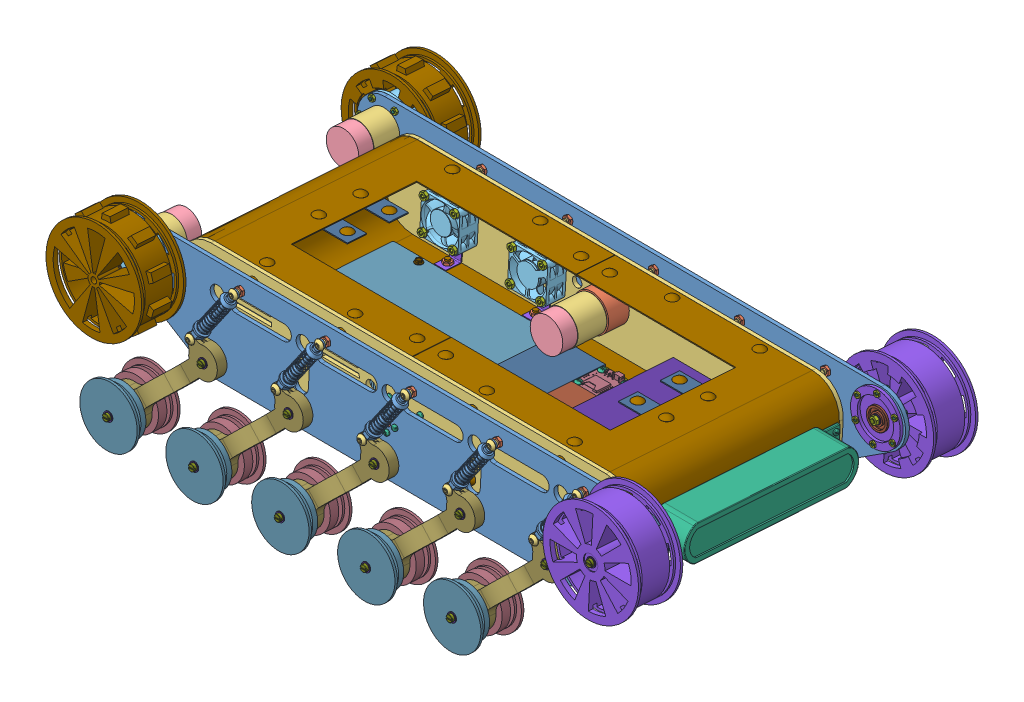
SolidWorks assembly Ensamble_Detallado_2, configuration Predeterminado. Lengths in mm. (continued)
Mates (geometry in assembly coordinates): (continued)
- Coincidente9464: coincident anti-aligned: plane of Perfil_IzquierdoV2.2-1 through (258.4555 -33.6114 -539.3761) normal (0.005872 -0.060029 -0.998179); plane of Acople-1 through (68.465 -3.1497 -542.3256) normal (-0.005872 0.060029 0.998179)
- Concéntrica118160: concentric aligned: cylinder of Perfil_IzquierdoV2.2-1 through (76.4414 -2.9112 -538.2857) axis (0.005872 -0.060029 -0.998179) radius 1.5; cylinder of Acople-1 through (76.4179 -2.6711 -534.293) axis (0.005872 -0.060029 -0.998179) radius 1.5
- Distancia1: distance = 0.55 mm anti-aligned: plane of Motor_4-2/Motor_1-1 through (68.5387 -3.9031 -554.8528) normal (-0.005872 0.060029 0.998179); plane of Acople-1 through (68.5355 -3.8701 -554.3038) normal (0.005872 -0.060029 -0.998179)
- Concéntrica118161: concentric aligned: cylinder of Motor_4-2/Motor_1-1 through (68.5387 -3.9031 -554.8528) axis (0.005872 -0.060029 -0.998179) radius 6; cylinder of Pared_chasis-2 through (68.5504 -4.0231 -556.8491) axis (0.005872 -0.060029 -0.998179) radius 6
- Coincidente9466: coincident anti-aligned: plane of Motor_4-2/Motor_1-1 through (67.8758 2.689 -561.264) normal (-0.005872 0.060029 0.998179); plane of Pared_chasis-2 through (275.5675 -9.2966 -559.3215) normal (0.005872 -0.060029 -0.998179)
- Concéntrica118165: concentric aligned: cylinder of Perfil_IzquierdoV2.2-1 through (60.4417 -2.908 -538.38) axis (0.005872 -0.060029 -0.998179) radius 1.5; cylinder of Acople-1 through (60.4182 -2.6679 -534.3873) axis (0.005872 -0.060029 -0.998179) radius 1.5
- Concéntrica118166: concentric anti-aligned: cylinder of Pared_chasis-2 through (76.058 16.8009 -558.0573) axis (0.005872 -0.060029 -0.998179) radius 1.5; cylinder of pan head tapping screw_am-43 through (76.0451 16.9329 -555.8613) axis (-0.005872 0.060029 0.998179) radius 1.5
- Coincidente9468: coincident anti-aligned: plane of Pared_chasis-2 through (275.544 -9.0565 -555.3288) normal (-0.005872 0.060029 0.998179); plane of pan head tapping screw_am-43 through (77.4539 14.3785 -557.9034) normal (0.005872 -0.060029 -0.998179)
- Concéntrica118167: concentric anti-aligned: cylinder of Perfil_IzquierdoV2.2-1 through (76.4414 -2.9112 -538.2857) axis (0.005872 -0.060029 -0.998179) radius 1.5; cylinder of pan head tapping screw_am-44 through (76.4285 -2.7792 -536.0897) axis (-0.005872 0.060029 0.998179) radius 1.5
- Coincidente9469: coincident anti-aligned: plane of Perfil_IzquierdoV2.2-1 through (258.432 -33.3713 -535.3834) normal (-0.005872 0.060029 0.998179); plane of pan head tapping screw_am-44 through (77.8372 -5.3336 -538.1318) normal (0.005872 -0.060029 -0.998179)
- Concéntrica118168: concentric aligned: cylinder of pan head tapping screw_am-44 through (76.4285 -2.7792 -536.0897) axis (-0.005872 0.060029 0.998179) radius 1.5; cylinder of hex nut style 1_am-64 through (76.4907 -3.4155 -546.6704) axis (-0.005872 0.060029 0.998179) radius 1.25
- Coincidente9470: coincident anti-aligned: plane of Acople-1 through (68.4767 -3.2698 -544.322) normal (0.005872 -0.060029 -0.998179); plane of hex nut style 1_am-64 through (80.2996 0.6768 -544.4898) normal (-0.005872 0.060029 0.998179)
- Paralelo35: parallel aligned: plane of Perfil_IzquierdoV2.2-1 through (-191.5245 49.7885 -543.0313) normal (0.000558 0.998197 -0.060026); plane of Pared_chasis-2 through (275.5742 44.8461 -558.5702) normal (0.000558 0.998197 -0.060026)
- Concéntrica118175: concentric anti-aligned: cylinder of Acople-1 through (68.5089 1.4211 -549.613) axis (-0.000558 -0.998197 0.060026) radius 1.5; cylinder of socket set screw cup point_ai-2 through (68.516 14.0982 -550.3753) axis (0.000558 0.998197 -0.060026) radius 1.5875
- Coincidente9473: coincident anti-aligned: plane of Ensamble_internoV1.1-1/ChasisV1.7-1 through (275.5809 14.6601 -560.7622) normal (-0.005872 0.060029 0.998179); plane of Pared_chasis-2 through (275.5675 -9.2966 -559.3215) normal (0.005872 -0.060029 -0.998179)
- Coincidente9474: coincident aligned: circle of Ensamble_internoV1.1-1/ChasisV1.7-1; circle of Pared_chasis-2
- Coincidente9477: coincident anti-aligned: plane of Pieza_union_chasis-3 through (-0.4051 43.6643 -564.1299) normal (-0.005872 0.060029 0.998179); plane of Pared_chasis-2 through (275.5675 -9.2966 -559.3215) normal (0.005872 -0.060029 -0.998179)
- Concéntrica118176: concentric aligned: circle of Pieza_union_chasis-3; cylinder of Pared_chasis-2 through (-0.4635 32.2862 -553.4277) axis (0.005872 -0.060029 -0.998179) radius 2.5
- Concéntrica118177: concentric anti-aligned: cylinder of round head bolt_ai-12 through (-0.4438 32.0846 -556.78) axis (-0.005872 0.060029 0.998179) radius 2.413; cylinder of Pared_chasis-2 through (-0.4635 32.2862 -553.4277) axis (0.005872 -0.060029 -0.998179) radius 2.5
- Coincidente9479: coincident anti-aligned: plane of round head bolt_ai-12 through (5.3374 31.9281 -559.383) normal (0.005872 -0.060029 -0.998179); plane of Pared_chasis-2 through (275.544 -9.0565 -555.3288) normal (-0.005872 0.060029 0.998179)
- Concéntrica118179: concentric anti-aligned: cylinder of hex nut jam_am-22 through (161.6055 -26.9975 -661.0978) axis (-0.000136 -0.06003 -0.998197) radius 2.1; cylinder of Pieza_union_chasis-9 through (-0.3972 -26.5933 -560.9065) axis (-0.005872 0.060029 0.998179) radius 2.5
- Coincidente9484: coincident anti-aligned: plane of Pared_chasis-2 through (275.5675 -9.2966 -559.3215) normal (0.005872 -0.060029 -0.998179); plane of Pieza_union_chasis-7 through (229.5909 43.6172 -562.7741) normal (-0.005872 0.060029 0.998179)
- Concéntrica118183: concentric anti-aligned: cylinder of Pared_chasis-2 through (229.5325 32.2391 -552.072) axis (0.005872 -0.060029 -0.998179) radius 2.5; cylinder of Pieza_union_chasis-7 through (229.5971 31.5788 -563.0519) axis (-0.005872 0.060029 0.998179) radius 2.5
- Concéntrica118184: concentric anti-aligned: cylinder of Ensamble_internoV1.1-1/ChasisV1.7-1 through (229.6462 -39.8004 -566.7736) axis (-0.000029 0.998197 -0.06003) radius 2.5; cylinder of Pieza_union_chasis-7 through (229.6435 50.0643 -572.1779) axis (0.000029 -0.998197 0.06003) radius 2.5
- Coincidente9485: coincident anti-aligned: plane of hex nut jam_am-33 through (229.9097 26.979 -562.7735) normal (-0.005872 0.060029 0.998179); plane of Pieza_union_chasis-7 through (229.5967 43.5572 -563.7723) normal (0.005872 -0.060029 -0.998179)
- Concéntrica118185: concentric aligned: cylinder of Pared_chasis-2 through (229.5325 32.2391 -552.072) axis (0.005872 -0.060029 -0.998179) radius 2.5; cylinder of hex nut jam_am-33 through (229.5971 31.5788 -563.0519) axis (0.005872 -0.060029 -0.998179) radius 2.1
- Coincidente9486: coincident anti-aligned: plane of Pared_chasis-2 through (275.544 -9.0565 -555.3288) normal (-0.005872 0.060029 0.998179); plane of round head bolt_ai-33 through (235.3334 31.881 -558.0272) normal (0.005872 -0.060029 -0.998179)
- Concéntrica118186: concentric anti-aligned: cylinder of Pared_chasis-2 through (229.5325 32.2391 -552.072) axis (0.005872 -0.060029 -0.998179) radius 2.5; cylinder of round head bolt_ai-33 through (229.5522 32.0375 -555.4242) axis (-0.005872 0.060029 0.998179) radius 2.413
- Coincidente9487: coincident anti-aligned: plane of Ensamble_internoV1.1-1/ChasisV1.7-1 through (-137.1798 31.8418 -774.6065) normal (-0.000029 0.998197 -0.06003); plane of round head bolt_ai-32 through (235.4095 44.0483 -571.8161) normal (0.000029 -0.998197 0.06003)
- Concéntrica118187: concentric aligned: cylinder of Ensamble_internoV1.1-1/ChasisV1.7-1 through (229.6462 -39.8004 -566.7736) axis (-0.000029 0.998197 -0.06003) radius 2.5; cylinder of round head bolt_ai-32 through (229.6436 46.685 -571.9747) axis (-0.000029 0.998197 -0.06003) radius 2.413
- Coincidente9488: coincident anti-aligned: plane of hex nut jam_am-32 through (229.9564 41.8021 -576.2976) normal (-0.000029 0.998197 -0.06003); plane of Pieza_union_chasis-7 through (235.6906 41.6008 -579.648) normal (0.000029 -0.998197 0.06003)
- Concéntrica118188: concentric aligned: cylinder of round head bolt_ai-32 through (229.6436 46.685 -571.9747) axis (-0.000029 0.998197 -0.06003) radius 2.413; cylinder of hex nut jam_am-32 through (229.6438 39.3836 -571.5356) axis (-0.000029 0.998197 -0.06003) radius 2.1
- Tangente1: tangent aligned: cylinder of Acople-1 through (68.5355 -3.8701 -554.3038) axis (-0.005872 0.060029 0.998179) radius 5; plane of socket set screw cup point_ai-2 through (68.5089 1.4211 -549.613) normal (0.000558 0.998197 -0.060026)
- Coincidente9489: coincident anti-aligned: plane of Ensamble_internoV1.1-1/ChasisV1.7-1 through (306.8142 -21.8912 -768.7633) normal (0.999983 0.000382 0.005859); plane of Soporte_zed-1 through (305.7303 18.7868 -586.4375) normal (-0.999983 -0.000382 -0.005859)
- Concéntrica118193: concentric anti-aligned: cylinder of Soporte_zed-1 through (308.6187 9.2915 -566.7568) axis (-0.999983 -0.000382 -0.005859) radius 1.5; cylinder of pan head tapping screw_am-57 through (310.8186 9.2924 -566.7439) axis (0.999983 0.000382 0.005859) radius 1.5
- Coincidente9492: coincident anti-aligned: plane of Soporte_zed-1 through (308.7833 0.6233 -594.2856) normal (0.999983 0.000382 0.005859); plane of pan head tapping screw_am-57 through (308.6257 11.7436 -568.1086) normal (-0.999983 -0.000382 -0.005859)
- Concéntrica118194: concentric anti-aligned: cylinder of Soporte_zed-1 through (308.6191 -4.6832 -565.9164) axis (-0.999983 -0.000382 -0.005859) radius 1.5; cylinder of pan head tapping screw_am-56 through (310.819 -4.6824 -565.9035) axis (0.999983 0.000382 0.005859) radius 1.5
- Coincidente9493: coincident anti-aligned: plane of Soporte_zed-1 through (308.7833 0.6233 -594.2856) normal (0.999983 0.000382 0.005859); plane of pan head tapping screw_am-56 through (308.6261 -2.2312 -567.2682) normal (-0.999983 -0.000382 -0.005859)
- Concéntrica118195: concentric anti-aligned: cylinder of Soporte_zed-1 through (309.7754 -2.5341 -763.3981) axis (-0.999983 -0.000382 -0.005859) radius 1.5; cylinder of pan head tapping screw_am-55 through (311.9754 -2.5333 -763.3853) axis (0.999983 0.000382 0.005859) radius 1.5
- Coincidente9494: coincident anti-aligned: plane of Soporte_zed-1 through (309.6112 -7.8407 -735.0289) normal (0.999983 0.000382 0.005859); plane of pan head tapping screw_am-55 through (309.7824 -0.0821 -764.7499) normal (-0.999983 -0.000382 -0.005859)
- Concéntrica118196: concentric anti-aligned: cylinder of Soporte_zed-1 through (309.7758 -16.5089 -762.5577) axis (-0.999983 -0.000382 -0.005859) radius 1.5; cylinder of pan head tapping screw_am-54 through (311.9758 -16.5081 -762.5448) axis (0.999983 0.000382 0.005859) radius 1.5
- Coincidente9495: coincident aligned: plane of Soporte_zed-1 through (309.6112 -7.8407 -735.0289) normal (0.999983 0.000382 0.005859); circle of pan head tapping screw_am-54
- Concéntrica118197: concentric anti-aligned: cylinder of pan head tapping screw_am-57 through (310.8186 9.2924 -566.7439) axis (0.999983 0.000382 0.005859) radius 1.5; cylinder of hex nut style 1_am-70 through (304.6187 9.29 -566.7802) axis (-0.999983 -0.000382 -0.005859) radius 1.25
- Coincidente9496: coincident anti-aligned: plane of Ensamble_internoV1.1-1/ChasisV1.7-1 through (305.8142 -21.8916 -768.7692) normal (-0.999983 -0.000382 -0.005859); plane of hex nut style 1_am-70 through (304.6117 4.0092 -565.243) normal (0.999983 0.000382 0.005859)
- Concéntrica118198: concentric anti-aligned: cylinder of pan head tapping screw_am-56 through (310.819 -4.6824 -565.9035) axis (0.999983 0.000382 0.005859) radius 1.5; cylinder of hex nut style 1_am-71 through (304.6192 -4.6848 -565.9398) axis (-0.999983 -0.000382 -0.005859) radius 1.25
- Coincidente9497: coincident anti-aligned: plane of Ensamble_internoV1.1-1/ChasisV1.7-1 through (305.8142 -21.8916 -768.7692) normal (-0.999983 -0.000382 -0.005859); plane of hex nut style 1_am-71 through (304.6122 -9.9656 -564.4025) normal (0.999983 0.000382 0.005859)
- Concéntrica118199: concentric anti-aligned: cylinder of pan head tapping screw_am-55 through (311.9754 -2.5333 -763.3853) axis (0.999983 0.000382 0.005859) radius 1.5; cylinder of hex nut style 1_am-68 through (305.7755 -2.5357 -763.4216) axis (-0.999983 -0.000382 -0.005859) radius 1.25
- Coincidente9498: coincident anti-aligned: plane of Ensamble_internoV1.1-1/ChasisV1.7-1 through (305.8142 -21.8916 -768.7692) normal (-0.999983 -0.000382 -0.005859); plane of hex nut style 1_am-68 through (305.7685 -7.8165 -761.8843) normal (0.999983 0.000382 0.005859)
- Concéntrica118200: concentric anti-aligned: cylinder of pan head tapping screw_am-54 through (311.9758 -16.5081 -762.5448) axis (0.999983 0.000382 0.005859) radius 1.5; cylinder of hex nut style 1_am-69 through (305.7759 -16.5104 -762.5812) axis (-0.999983 -0.000382 -0.005859) radius 1.25
- Coincidente9499: coincident anti-aligned: plane of Ensamble_internoV1.1-1/ChasisV1.7-1 through (305.8142 -21.8916 -768.7692) normal (-0.999983 -0.000382 -0.005859); plane of hex nut style 1_am-69 through (305.7689 -21.7912 -761.0439) normal (0.999983 0.000382 0.005859)
- Coincidente9501: coincident anti-aligned: plane of Ensamble_internoV1.1-1/ChasisV1.7-1 through (306.8142 -21.8912 -768.7633) normal (0.999983 0.000382 0.005859); plane of ZED.step-3 through (305.7833 0.6222 -594.3032) normal (-0.999983 -0.000382 -0.005859)
- Concéntrica118201: concentric aligned: cylinder of Soporte_zed-1 through (306.6112 -7.8419 -735.0465) axis (0.999983 0.000382 0.005859) radius 17; cone of ZED.step-3 through (306.5112 -7.8419 -735.0471) axis (0.999983 0.000382 0.005859)
- Concéntrica118202: concentric aligned: cylinder of Soporte_zed-1 through (305.7833 0.6222 -594.3032) axis (0.999983 0.000382 0.005859) radius 17; cone of ZED.step-3 through (305.6833 0.6221 -594.3038) axis (0.999983 0.000382 0.005859)
- Concéntrica118203: concentric aligned: cylinder of Soporte_zed-1 through (306.6112 -7.8419 -735.0465) axis (0.999983 0.000382 0.005859) radius 17; cylinder of Tapazed-1 through (338.0107 -7.8299 -734.8625) axis (0.999983 0.000382 0.005859) radius 17
- Concéntrica118204: concentric aligned: cylinder of Soporte_zed-1 through (305.7833 0.6222 -594.3032) axis (0.999983 0.000382 0.005859) radius 17; cylinder of Tapazed-1 through (337.1828 0.6342 -594.1192) axis (0.999983 0.000382 0.005859) radius 17
- Coincidente9503: coincident anti-aligned: plane of ZED.step-3 through (338.0107 -7.8299 -734.8625) normal (0.999983 0.000382 0.005859); plane of Tapazed-1 through (337.1349 15.8796 -586.9451) normal (-0.999983 -0.000382 -0.005859)
- Concéntrica1182071: concentric aligned: cylinder of fan-1 through (16.1953 17.9752 -582.5238) axis (-0.005872 0.060029 0.998179) radius 2; cylinder of fillister head tapping screw_ai-1 through (16.0403 19.5593 -556.1843) axis (-0.005872 0.060029 0.998179) radius 1.9177
- Concéntrica118208: concentric aligned: cylinder of fan-1 through (-15.8042 17.9696 -582.7117) axis (-0.005872 0.060029 0.998179) radius 2; cylinder of fillister head tapping screw_ai-2 through (-15.9591 19.5536 -556.3721) axis (-0.005872 0.060029 0.998179) radius 1.9177
- Concéntrica118209: concentric aligned: cylinder of fan-1 through (-15.8098 -13.9727 -580.7908) axis (-0.005872 0.060029 0.998179) radius 2; cylinder of fillister head tapping screw_ai-6 through (-15.9647 -12.3887 -554.4512) axis (-0.005872 0.060029 0.998179) radius 1.9177
- Concéntrica118210: concentric aligned: cylinder of fan-1 through (16.1896 -13.967 -580.6029) axis (-0.005872 0.060029 0.998179) radius 2; cylinder of fillister head tapping screw_ai-7 through (16.0347 -12.383 -554.2633) axis (-0.005872 0.060029 0.998179) radius 1.9177
- Coincidente9506: coincident anti-aligned: plane of fan-1 through (16.1896 -13.967 -580.6029) normal (0.005872 -0.060029 -0.998179); plane of hex nut style 1 gradeab_bsi-7 through (16.9128 21.9456 -582.7584) normal (-0.005872 0.060029 0.998179)
- Concéntrica118211: concentric anti-aligned: cylinder of hex nut style 1 gradeab_bsi-7 through (16.1953 17.9752 -582.5238) axis (0.005872 -0.060029 -0.998179) radius 1.65; cylinder of fillister head tapping screw_ai-1 through (16.0403 19.5593 -556.1843) axis (-0.005872 0.060029 0.998179) radius 1.9177
- Concéntrica118212: concentric anti-aligned: cylinder of hex nut style 1 gradeab_bsi-8 through (16.1896 -13.967 -580.6029) axis (0.005872 -0.060029 -0.998179) radius 1.65; cylinder of fillister head tapping screw_ai-7 through (16.0347 -12.383 -554.2633) axis (-0.005872 0.060029 0.998179) radius 1.9177
- Coincidente9507: coincident anti-aligned: plane of fan-1 through (16.1896 -13.967 -580.6029) normal (0.005872 -0.060029 -0.998179); plane of hex nut style 1 gradeab_bsi-8 through (19.3936 -16.4247 -580.4362) normal (-0.005872 0.060029 0.998179)
- Coincidente9508: coincident anti-aligned: plane of fan-1 through (16.1896 -13.967 -580.6029) normal (0.005872 -0.060029 -0.998179); plane of hex nut style 1 gradeab_bsi-5 through (-12.5278 20.3326 -582.8345) normal (-0.005872 0.060029 0.998179)
- Concéntrica118213: concentric anti-aligned: cylinder of hex nut style 1 gradeab_bsi-5 through (-15.8042 17.9696 -582.7117) axis (0.005872 -0.060029 -0.998179) radius 1.65; cylinder of fillister head tapping screw_ai-2 through (-15.9591 19.5536 -556.3721) axis (-0.005872 0.060029 0.998179) radius 1.9177
- Concéntrica118214: concentric aligned: circle of fan-1; cylinder of hex nut style 1 gradeab_bsi-6 through (-15.8098 -13.9727 -580.7908) axis (0.005872 -0.060029 -0.998179) radius 1.65
- Coincidente9509: coincident anti-aligned: plane of fan-1 through (16.1896 -13.967 -580.6029) normal (0.005872 -0.060029 -0.998179); plane of hex nut style 1 gradeab_bsi-6 through (-12.6058 -16.4304 -580.6241) normal (-0.005872 0.060029 0.998179)
- Concéntrica118215: concentric anti-aligned: cylinder of fan-2 through (-107.8172 18.1385 -580.7586) axis (0.005872 -0.060029 -0.998179) radius 3.5; cylinder of hex nut style 1 gradeab_bsi-1 through (-107.7838 17.7963 -586.4482) axis (-0.005872 0.060029 0.998179) radius 1.65
- Concéntrica118216: concentric aligned: cylinder of fan-2 through (-107.8229 -13.8038 -578.8376) axis (0.005872 -0.060029 -0.998179) radius 3.5; cylinder of hex nut style 1 gradeab_bsi-2 through (-107.8082 -13.9539 -581.3331) axis (0.005872 -0.060029 -0.998179) radius 1.65
- Concéntrica118217: concentric aligned: cylinder of fan-2 through (-75.8178 18.1442 -580.5707) axis (0.005872 -0.060029 -0.998179) radius 3.5; cylinder of hex nut style 1 gradeab_bsi-4 through (-75.8031 17.9941 -583.0661) axis (0.005872 -0.060029 -0.998179) radius 1.65
- Concéntrica118218: concentric aligned: cylinder of fan-2 through (-75.8234 -13.7981 -578.6497) axis (0.005872 -0.060029 -0.998179) radius 3.5; cylinder of hex nut style 1 gradeab_bsi-3 through (-75.8088 -13.9482 -581.1452) axis (0.005872 -0.060029 -0.998179) radius 1.65
- Concéntrica118219: concentric anti-aligned: cylinder of fan-2 through (-107.92 19.189 -563.2904) axis (0.005872 -0.060029 -0.998179) radius 2; cylinder of fillister head tapping screw_ai-3 through (-107.9575 19.5725 -556.9145) axis (-0.005872 0.060029 0.998179) radius 1.9177
- Concéntrica118220: concentric anti-aligned: cylinder of fan-2 through (-75.9205 19.1947 -563.1025) axis (0.005872 -0.060029 -0.998179) radius 2; cylinder of fillister head tapping screw_ai-4 through (-75.9581 19.5781 -556.7266) axis (-0.005872 0.060029 0.998179) radius 1.9177
- Concéntrica118221: concentric anti-aligned: cylinder of fan-2 through (-107.9256 -12.7533 -561.3695) axis (0.005872 -0.060029 -0.998179) radius 2; cylinder of fillister head tapping screw_ai-8 through (-107.9631 -12.3698 -554.9935) axis (-0.005872 0.060029 0.998179) radius 1.9177
- Concéntrica118222: concentric anti-aligned: cylinder of fan-2 through (-75.9262 -12.7476 -561.1816) axis (0.005872 -0.060029 -0.998179) radius 2; cylinder of fillister head tapping screw_ai-5 through (-75.9637 -12.3642 -554.8056) axis (-0.005872 0.060029 0.998179) radius 1.9177
- Coincidente9510: coincident anti-aligned: plane of fan-2 through (-107.9256 -12.7533 -561.3695) normal (-0.005872 0.060029 0.998179); plane of Pared_chasis-2 through (275.5675 -9.2966 -559.3215) normal (0.005872 -0.060029 -0.998179)
- Concéntrica118223: concentric anti-aligned: cylinder of fan-2 through (-107.92 19.189 -563.2904) axis (0.005872 -0.060029 -0.998179) radius 2; cylinder of Pared_chasis-2 through (-107.8848 18.8288 -569.2795) axis (-0.005872 0.060029 0.998179) radius 2
- Coincidente9511: coincident anti-aligned: plane of Pared_chasis-2 through (275.544 -9.0565 -555.3288) normal (-0.005872 0.060029 0.998179); plane of fillister head tapping screw_ai-3 through (-107.9431 21.3434 -559.4128) normal (0.005872 -0.060029 -0.998179)
- Coincidente9512: coincident anti-aligned: plane of Pared_chasis-2 through (275.544 -9.0565 -555.3288) normal (-0.005872 0.060029 0.998179); plane of fillister head tapping screw_ai-8 through (-107.9488 -10.5989 -557.4919) normal (0.005872 -0.060029 -0.998179)
- Coincidente9513: coincident anti-aligned: plane of Pared_chasis-2 through (275.544 -9.0565 -555.3288) normal (-0.005872 0.060029 0.998179); plane of fillister head tapping screw_ai-4 through (-75.9437 21.349 -559.2249) normal (0.005872 -0.060029 -0.998179)
- Coincidente9514: coincident anti-aligned: plane of Pared_chasis-2 through (275.544 -9.0565 -555.3288) normal (-0.005872 0.060029 0.998179); plane of fillister head tapping screw_ai-5 through (-75.9493 -10.5933 -557.304) normal (0.005872 -0.060029 -0.998179)
- Coincidente9515: coincident anti-aligned: plane of fan-1 through (16.0722 -12.7665 -560.6393) normal (-0.005872 0.060029 0.998179); plane of Pared_chasis-2 through (275.5675 -9.2966 -559.3215) normal (0.005872 -0.060029 -0.998179)
- Concéntrica118224: concentric aligned: cylinder of fan-1 through (-15.8042 17.9696 -582.7117) axis (-0.005872 0.060029 0.998179) radius 2; cylinder of Pared_chasis-2 through (-15.8864 18.81 -568.7372) axis (-0.005872 0.060029 0.998179) radius 2
- Coincidente9516: coincident anti-aligned: plane of Pared_chasis-2 through (275.544 -9.0565 -555.3288) normal (-0.005872 0.060029 0.998179); plane of fillister head tapping screw_ai-2 through (-15.9447 21.3245 -558.8705) normal (0.005872 -0.060029 -0.998179)
- Coincidente9517: coincident anti-aligned: plane of Pared_chasis-2 through (275.544 -9.0565 -555.3288) normal (-0.005872 0.060029 0.998179); plane of fillister head tapping screw_ai-1 through (16.0547 21.3302 -558.6826) normal (0.005872 -0.060029 -0.998179)
- Coincidente9518: coincident anti-aligned: plane of Pared_chasis-2 through (275.544 -9.0565 -555.3288) normal (-0.005872 0.060029 0.998179); plane of fillister head tapping screw_ai-6 through (-15.9504 -10.6178 -556.9496) normal (0.005872 -0.060029 -0.998179)
- Coincidente9519: coincident anti-aligned: plane of Pared_chasis-2 through (275.544 -9.0565 -555.3288) normal (-0.005872 0.060029 0.998179); plane of fillister head tapping screw_ai-7 through (16.0491 -10.6121 -556.7617) normal (0.005872 -0.060029 -0.998179)
- Concéntrica118225: concentric aligned: cylinder of Motor_4-1/Motor_1-1 through (-191.7991 18.2215 -497.5552) axis (0.005872 -0.060029 -0.998179) radius 3; cylinder of Rueda_TraseraV1.2-1 through (-191.6758 16.9609 -518.5169) axis (0.005872 -0.060029 -0.998179) radius 33.5
- Concéntrica1182073: concentric aligned: cylinder of Perfil_IzquierdoV2.2-1 through (328.4512 22.4912 -538.331) axis (0.005872 -0.060029 -0.998179) radius 11; cylinder of instrument ball bearing_68_am-8 through (328.3506 23.5199 -521.2247) axis (0.005872 -0.060029 -0.998179) radius 11
- Coincidente9520: coincident anti-aligned: plane of Pieza_Fijacion-1 through (328.1431 22.6984 -545.358) normal (-0.005872 0.060029 0.998179); plane of instrument ball bearing_68_am-8 through (338.1183 26.738 -545.5423) normal (0.005872 -0.060029 -0.998179)
- Concéntrica1182075: concentric aligned: cylinder of Rueda_FrenteV1.2-2 through (328.1664 25.4025 -489.9193) axis (0.005872 -0.060029 -0.998179) radius 4; cylinder of instrument ball bearing_68_am-8 through (328.3506 23.5199 -521.2247) axis (0.005872 -0.060029 -0.998179) radius 4
- Coincidente9522: coincident anti-aligned: plane of Rueda_FrenteV1.2-2 through (328.4512 22.4912 -538.331) normal (0.005872 -0.060029 -0.998179); plane of instrument ball bearing_68_am-8 through (333.9389 25.1518 -538.4587) normal (-0.005872 0.060029 0.998179)
- Concéntrica1182076: concentric anti-aligned: cylinder of Rueda_FrenteV1.2-2 through (328.1723 25.3425 -490.9174) axis (-0.005872 0.060029 0.998179) radius 7.5; cylinder of Pasador-3 through (328.231 24.7422 -500.8992) axis (0.005872 -0.060029 -0.998179) radius 4
- Concéntrica1182077: concentric anti-aligned: cylinder of Pasador-3 through (328.231 24.7422 -500.8992) axis (0.005872 -0.060029 -0.998179) radius 2; cylinder of cheese head screw_as-4 through (328.1524 25.5466 -487.5236) axis (-0.005872 0.060029 0.998179) radius 2
- Concéntrica1182078: concentric anti-aligned: cylinder of cheese head screw_as-4 through (328.1524 25.5466 -487.5236) axis (-0.005872 0.060029 0.998179) radius 2; circle of plain washer - normal_as-5
- Coincidente9523: coincident anti-aligned: plane of Rueda_FrenteV1.2-2 through (328.1723 25.3425 -490.9174) normal (-0.005872 0.060029 0.998179); plane of plain washer - normal_as-5 through (326.0262 25.2129 -490.9223) normal (0.005872 -0.060029 -0.998179)
- Coincidente9524: coincident anti-aligned: plane of cheese head screw_as-4 through (328.1779 21.8969 -489.9087) normal (0.005872 -0.060029 -0.998179); plane of plain washer - normal_as-5 through (326.0215 25.261 -490.1237) normal (-0.005872 0.060029 0.998179)
- Concéntrica1182080: concentric anti-aligned: cylinder of cheese head screw_as-4 through (328.1524 25.5466 -487.5236) axis (-0.005872 0.060029 0.998179) radius 2; cylinder of hex nut style 1_am-72 through (328.497 22.0229 -546.1168) axis (0.005872 -0.060029 -0.998179) radius 1.65
- Coincidente9527: coincident aligned: plane of Rueda_Resorte2V1.3-13 through (188.9664 -93.9124 -529.6466) normal (0.005872 -0.060029 -0.998179); plane of Rueda_TraseraV1.2-1 through (-191.5583 15.7604 -538.4805) normal (0.005872 -0.060029 -0.998179)
- Concéntrica1182087: concentric aligned: cylinder of Rueda_TraseraV1.2-1 through (-191.7932 18.1615 -498.5534) axis (-0.925273 -0.378905 0.017344) radius 1.5; cylinder of socket set screw cup point_ai-3 through (-209.0958 11.076 -498.229) axis (-0.925273 -0.378905 0.017344) radius 1.5875
- Tangente2: tangent aligned: cylinder of Rueda_TraseraV1.2-1 through (-191.5583 15.7604 -538.4805) axis (-0.005872 0.060029 0.998179) radius 6; plane of socket set screw cup point_ai-3 through (-197.3448 15.8881 -498.4493) normal (-0.925273 -0.378905 0.017344)
- Paralelo39: parallel aligned: plane of Perfil_IzquierdoV2.2-1 through (-191.5245 49.7885 -543.0313) normal (0.000558 0.998197 -0.060026); plane of Motor_4-1/Motor_1-1 through (-189.9977 20.6168 -497.6886) normal (0.000558 0.998197 -0.060026)
- Concéntrica1182089: concentric anti-aligned: circle of instrument ball bearing_68_am-8; circle of Tapa_Rueda_Delantera-1
- Coincidente9529: coincident anti-aligned: plane of instrument ball bearing_68_am-8 through (336.4578 26.3731 -538.5173) normal (-0.005872 0.060029 0.998179); plane of Tapa_Rueda_Delantera-1 through (328.4512 22.4912 -538.331) normal (0.005872 -0.060029 -0.998179)
- Concéntrica1182090: concentric anti-aligned: cylinder of pan head tapping screw_am-20 through (328.8149 45.7585 -536.5222) axis (-0.005872 0.060029 0.998179) radius 1.5; cylinder of Tapa_Rueda_Delantera-1 through (328.8278 45.6265 -538.7182) axis (0.005872 -0.060029 -0.998179) radius 1.5
- Coincidente9530: coincident anti-aligned: plane of pan head tapping screw_am-20 through (330.2891 48.0111 -538.8531) normal (0.005872 -0.060029 -0.998179); plane of Tapa_Rueda_Delantera-1 through (328.4454 22.5512 -537.3328) normal (-0.005872 0.060029 0.998179)
- Coincidente9531: coincident aligned: plane of instrument ball bearing_68_am-8 through (332.3607 23.9465 -545.4083) normal (0.005872 -0.060029 -0.998179); plane of Pasador-3 through (328.4923 22.071 -545.3182) normal (0.005872 -0.060029 -0.998179)
- Concéntrica1182091: concentric anti-aligned: cylinder of cheese head screw_as-4 through (328.1524 25.5466 -487.5236) axis (-0.005872 0.060029 0.998179) radius 2; cylinder of plain washer - normal_as-6 through (328.497 22.0229 -546.1168) axis (0.005872 -0.060029 -0.998179) radius 2.15
- Coincidente9532: coincident anti-aligned: plane of instrument ball bearing_68_am-8 through (332.3607 23.9465 -545.4083) normal (0.005872 -0.060029 -0.998179); plane of plain washer - normal_as-6 through (326.3462 21.9414 -545.3231) normal (-0.005872 0.060029 0.998179)
- Coincidente9533: coincident anti-aligned: plane of hex nut style 1_am-72 through (328.7641 26.0484 -546.3573) normal (-0.005872 0.060029 0.998179); plane of plain washer - normal_as-6 through (326.3509 21.8933 -546.1216) normal (0.005872 -0.060029 -0.998179)
- Concéntrica1182094: concentric aligned: cylinder of Perfil_IzquierdoV2.2-1 through (272.3532 35.9869 -549.4908) axis (-0.005872 0.060029 0.998179) radius 2; cylinder of socket button head cap screw_am-4 through (272.2343 37.2025 -529.2777) axis (-0.005872 0.060029 0.998179) radius 2.5
- Coincidente9535: coincident anti-aligned: plane of Resorte-1 through (272.2505 37.0374 -532.0227) normal (-0.005872 0.060029 0.998179); plane of socket button head cap screw_am-4 through (274.739 37.2769 -532.0224) normal (0.005872 -0.060029 -0.998179)
- Concéntrica1182095: concentric aligned: cylinder of socket button head cap screw_am-4 through (272.2343 37.2025 -529.2777) axis (-0.005872 0.060029 0.998179) radius 2.5; cylinder of hex nut jam_am-68 through (272.3338 36.185 -546.1968) axis (-0.005872 0.060029 0.998179) radius 2.1
- Coincidente9536: coincident anti-aligned: plane of Perfil_IzquierdoV2.2-1 through (258.4555 -33.6114 -539.3761) normal (0.005872 -0.060029 -0.998179); plane of hex nut jam_am-68 through (272.0407 40.9492 -543.7801) normal (-0.005872 0.060029 0.998179)
- Concéntrica1182096: concentric aligned: cylinder of socket button head cap screw_am-4 through (272.2343 37.2025 -529.2777) axis (-0.005872 0.060029 0.998179) radius 2.5; cylinder of hex nut jam_am-67 through (272.2945 36.5872 -539.509) axis (-0.005872 0.060029 0.998179) radius 2.1
- Coincidente9537: coincident anti-aligned: plane of Perfil_IzquierdoV2.2-1 through (258.432 -33.3713 -535.3834) normal (-0.005872 0.060029 0.998179); plane of hex nut jam_am-67 through (272.0172 41.1893 -539.7874) normal (0.005872 -0.060029 -0.998179)
- Concéntrica1182097: concentric anti-aligned: cylinder of Perfil_IzquierdoV2.2-2 through (273.8276 20.9137 -800.1337) axis (-0.005872 0.060029 0.998179) radius 2; cylinder of socket button head cap screw_am-7 through (273.8526 20.6586 -804.3759) axis (0.005872 -0.060029 -0.998179) radius 2.5
- Coincidente9538: coincident anti-aligned: plane of Resorte-2 through (273.8364 20.8237 -801.6309) normal (0.005872 -0.060029 -0.998179); plane of socket button head cap screw_am-7 through (276.3249 20.586 -801.602) normal (-0.005872 0.060029 0.998179)
- Concéntrica1182098: concentric aligned: cylinder of Resorte-2 through (273.8364 20.8237 -801.6309) axis (-0.005872 0.060029 0.998179) radius 2.4; cylinder of Perfil_IzquierdoV2.2-2 through (273.8276 20.9137 -800.1337) axis (-0.005872 0.060029 0.998179) radius 2
- Concéntrica1182099: concentric anti-aligned: cylinder of hex nut jam_am-66 through (273.7689 21.514 -790.1519) axis (-0.005872 0.060029 0.998179) radius 2.1; cylinder of socket button head cap screw_am-7 through (273.8526 20.6586 -804.3759) axis (0.005872 -0.060029 -0.998179) radius 2.5
- Coincidente9540: coincident anti-aligned: plane of Perfil_IzquierdoV2.2-2 through (259.9064 -48.4445 -786.0262) normal (-0.005872 0.060029 0.998179); plane of hex nut jam_am-66 through (273.4916 26.1161 -790.4302) normal (0.005872 -0.060029 -0.998179)
- Concéntrica1182100: concentric anti-aligned: cylinder of hex nut jam_am-65 through (273.8082 21.1118 -796.8397) axis (-0.005872 0.060029 0.998179) radius 2.1; cylinder of socket button head cap screw_am-7 through (273.8526 20.6586 -804.3759) axis (0.005872 -0.060029 -0.998179) radius 2.5
- Coincidente9541: coincident anti-aligned: plane of Perfil_IzquierdoV2.2-2 through (259.9299 -48.6846 -790.0189) normal (0.005872 -0.060029 -0.998179); plane of hex nut jam_am-65 through (273.5151 25.8759 -794.423) normal (-0.005872 0.060029 0.998179)
- Coincidente9542: coincident anti-aligned: plane of Perfil_IzquierdoV2.2-1 through (258.432 -33.3713 -535.3834) normal (-0.005872 0.060029 0.998179); plane of instrument ball bearing_68_am-11 through (255.9175 -38.1776 -535.1091) normal (0.005872 -0.060029 -0.998179)
- Coincidente9543: coincident anti-aligned: plane of Pieza_ResorteV1.5-6 through (248.3803 -32.9713 -528.4538) normal (0.005872 -0.060029 -0.998179); plane of instrument ball bearing_68_am-11 through (257.3925 -38.7254 -528.0547) normal (-0.005872 0.060029 0.998179)
- Concéntrica1182102: concentric aligned: cylinder of Pieza_ResorteV1.5-6 through (248.3891 -33.0613 -529.9511) axis (-0.005872 0.060029 0.998179) radius 2; cylinder of instrument ball bearing_68_am-11 through (248.522 -34.4202 -552.5474) axis (-0.005872 0.060029 0.998179) radius 4
- Coincidente9544: coincident aligned: plane of instrument ball bearing_68_am-11 through (252.002 -35.2837 -528.2934) normal (-0.005872 0.060029 0.998179); plane of Tubo_Pata-1 through (248.3803 -32.9713 -528.4538) normal (-0.005872 0.060029 0.998179)
- Concéntrica1182105: concentric anti-aligned: cylinder of Tubo_Pata-1 through (248.3803 -32.9713 -528.4538) axis (0.005872 -0.060029 -0.998179) radius 2; cylinder of cheese head screw_as-6 through (248.3339 -32.497 -520.5682) axis (-0.005872 0.060029 0.998179) radius 2
- Concéntrica1182107: concentric anti-aligned: cylinder of cheese head screw_as-6 through (248.3339 -32.497 -520.5682) axis (-0.005872 0.060029 0.998179) radius 2; cylinder of plain washer - normal_as-10 through (248.3538 -32.7011 -523.962) axis (0.005872 -0.060029 -0.998179) radius 2.15
- Coincidente9546: coincident anti-aligned: plane of Pieza_ResorteV1.5-6 through (254.0133 -38.2259 -523.5964) normal (-0.005872 0.060029 0.998179); plane of plain washer - normal_as-10 through (246.2077 -32.8307 -523.9668) normal (0.005872 -0.060029 -0.998179)
- Coincidente9547: coincident anti-aligned: plane of cheese head screw_as-6 through (248.3595 -36.1468 -522.9533) normal (0.005872 -0.060029 -0.998179); plane of plain washer - normal_as-10 through (246.203 -32.7827 -523.1683) normal (-0.005872 0.060029 0.998179)
- Concéntrica1182108: concentric anti-aligned: cylinder of cheese head screw_as-6 through (248.3339 -32.497 -520.5682) axis (-0.005872 0.060029 0.998179) radius 2; cylinder of hex nut style 1_am-101 through (248.4495 -33.6796 -540.2323) axis (0.005872 -0.060029 -0.998179) radius 1.65
- Concéntrica1182109: concentric anti-aligned: cylinder of Perfil_IzquierdoV2.2-1 through (248.4214 -33.3915 -535.4411) axis (0.005872 -0.060029 -0.998179) radius 4; cylinder of cheese head screw_as-6 through (248.3339 -32.497 -520.5682) axis (-0.005872 0.060029 0.998179) radius 2
- Concéntrica1182110: concentric anti-aligned: cylinder of instrument ball bearing_68_am-11 through (248.522 -34.4202 -552.5474) axis (-0.005872 0.060029 0.998179) radius 4; cylinder of Tubo_Pata-1 through (248.3803 -32.9713 -528.4538) axis (0.005872 -0.060029 -0.998179) radius 4
- Coincidente9549: coincident anti-aligned: plane of Perfil_IzquierdoV2.2-1 through (258.4555 -33.6114 -539.3761) normal (0.005872 -0.060029 -0.998179); plane of plain washer - normal_as-11 through (250.5055 -34.2431 -539.3849) normal (-0.005872 0.060029 0.998179)
- Concéntrica1182111: concentric anti-aligned: cylinder of cheese head screw_as-6 through (248.3339 -32.497 -520.5682) axis (-0.005872 0.060029 0.998179) radius 2; cylinder of plain washer - normal_as-11 through (248.4495 -33.6796 -540.2323) axis (0.005872 -0.060029 -0.998179) radius 2.15
- Coincidente9550: coincident anti-aligned: plane of hex nut style 1_am-101 through (248.2318 -29.6514 -540.4758) normal (-0.005872 0.060029 0.998179); plane of plain washer - normal_as-11 through (250.5102 -34.2911 -540.1834) normal (0.005872 -0.060029 -0.998179)
- Concéntrica1182112: concentric anti-aligned: cylinder of instrument ball bearing_68_am-7 through (250.061 -50.1537 -814.1702) axis (-0.005872 0.060029 0.998179) radius 4; cylinder of Perfil_IzquierdoV2.2-2 through (249.8957 -48.4647 -786.0839) axis (0.005872 -0.060029 -0.998179) radius 4
- Coincidente9551: coincident anti-aligned: plane of instrument ball bearing_68_am-7 through (246.089 -46.7555 -790.2164) normal (-0.005872 0.060029 0.998179); plane of Perfil_IzquierdoV2.2-2 through (259.9299 -48.6846 -790.0189) normal (0.005872 -0.060029 -0.998179)
- Concéntrica1182113: concentric anti-aligned: cylinder of Pieza_Resorte_2V1.5-1 through (249.9545 -49.065 -796.0657) axis (0.005872 -0.060029 -0.998179) radius 4; cylinder of instrument ball bearing_68_am-7 through (250.061 -50.1537 -814.1702) axis (-0.005872 0.060029 0.998179) radius 4
- Concéntrica1182114: concentric aligned: cylinder of Pieza_Resorte_2V1.5-1 through (249.9545 -49.065 -796.0657) axis (0.005872 -0.060029 -0.998179) radius 4; cylinder of cheese head screw_as-7 through (250.0067 -49.5992 -804.9495) axis (0.005872 -0.060029 -0.998179) radius 2
- Concéntrica1182115: concentric aligned: circle of Pieza_Resorte_2V1.5-1; cylinder of plain washer - normal_as-13 through (249.9914 -49.4432 -802.3542) axis (0.005872 -0.060029 -0.998179) radius 2.15
- Coincidente9552: coincident anti-aligned: plane of Pieza_Resorte_2V1.5-1 through (244.3273 -43.8704 -801.9212) normal (0.005872 -0.060029 -0.998179); plane of plain washer - normal_as-13 through (252.0474 -50.0067 -801.5068) normal (-0.005872 0.060029 0.998179)
- Coincidente9553: coincident anti-aligned: plane of cheese head screw_as-7 through (253.4674 -49.8502 -802.3093) normal (-0.005872 0.060029 0.998179); plane of plain washer - normal_as-13 through (252.0521 -50.0547 -802.3053) normal (0.005872 -0.060029 -0.998179)
- Concéntrica1182118: concentric aligned: cylinder of cheese head screw_as-7 through (250.0067 -49.5992 -804.9495) axis (0.005872 -0.060029 -0.998179) radius 2; cylinder of plain washer - normal_as-12 through (249.8957 -48.4647 -786.0839) axis (0.005872 -0.060029 -0.998179) radius 2.15
- Coincidente9556: coincident anti-aligned: plane of Perfil_IzquierdoV2.2-2 through (259.9064 -48.4445 -786.0262) normal (-0.005872 0.060029 0.998179); plane of plain washer - normal_as-12 through (247.7497 -48.5943 -786.0887) normal (0.005872 -0.060029 -0.998179)
- Concéntrica1182119: concentric aligned: cylinder of cheese head screw_as-7 through (250.0067 -49.5992 -804.9495) axis (0.005872 -0.060029 -0.998179) radius 2; cylinder of hex nut style 1_am-102 through (249.8722 -48.2246 -782.0912) axis (0.005872 -0.060029 -0.998179) radius 1.65
- Coincidente9557: coincident aligned: circle of hex nut style 1_am-102; plane of plain washer - normal_as-12 through (247.745 -48.5463 -785.2902) normal (-0.005872 0.060029 0.998179)
- Concéntrica1182120: concentric aligned: cylinder of Resorte-1 through (272.2622 36.9174 -534.019) axis (-0.005872 0.060029 0.998179) radius 4.15; cylinder of socket button head cap screw_am-4 through (272.2343 37.2025 -529.2777) axis (-0.005872 0.060029 0.998179) radius 2.5
- Coincidente9558: coincident anti-aligned: plane of Pieza_Resorte_2V1.5-1 through (249.9603 -49.125 -797.0639) normal (-0.005872 0.060029 0.998179); plane of instrument ball bearing_68_am-7 through (242.0326 -45.0904 -797.3531) normal (0.005872 -0.060029 -0.998179)
- Concéntrica1182123: concentric anti-aligned: cylinder of Pasador-2 through (190.4936 -109.5258 -789.2731) axis (0.005872 -0.060029 -0.998179) radius 4; cylinder of Rueda_Resorte2V1.3-15 through (190.5053 -109.6459 -791.2694) axis (-0.005872 0.060029 0.998179) radius 4
- Coincidente9559: coincident anti-aligned: plane of plain washer - normal_as-3 through (188.3437 -109.5375 -789.285) normal (0.005872 -0.060029 -0.998179); plane of Rueda_Resorte2V1.3-15 through (190.4936 -109.5258 -789.2731) normal (-0.005872 0.060029 0.998179)
- Coincidente9561: coincident aligned: plane of Pasador-2 through (190.4936 -109.5258 -789.2731) normal (-0.005872 0.060029 0.998179); plane of Rueda_Resorte2V1.3-15 through (190.4936 -109.5258 -789.2731) normal (-0.005872 0.060029 0.998179)
- Concéntrica1182124: concentric aligned: cylinder of Pasador-2 through (190.4936 -109.5258 -789.2731) axis (0.005872 -0.060029 -0.998179) radius 4; cylinder of Rueda_ResorteV1.3-19 through (190.7431 -112.0771 -831.6957) axis (0.005872 -0.060029 -0.998179) radius 4
- Coincidente9562: coincident anti-aligned: plane of Pieza_Resorte_2V1.5-1 through (202.7379 -87.6413 -819.57) normal (0.005872 -0.060029 -0.998179); plane of Rueda_ResorteV1.3-19 through (190.6639 -111.2667 -818.2203) normal (-0.005872 0.060029 0.998179)
- Coincidente9563: coincident anti-aligned: plane of Pieza_Resorte_2V1.5-1 through (202.6792 -87.041 -809.5882) normal (-0.005872 0.060029 0.998179); plane of Rueda_Resorte2V1.3-15 through (190.6052 -110.6664 -808.2385) normal (0.005872 -0.060029 -0.998179)
- Coincidente9564: coincident anti-aligned: plane of plain washer - normal_as-4 through (188.605 -112.2088 -833.704) normal (-0.005872 0.060029 0.998179); plane of Rueda_ResorteV1.3-19 through (190.7549 -112.1971 -833.692) normal (0.005872 -0.060029 -0.998179)
- Concéntrica1182125: concentric aligned: cylinder of cheese head screw_as-7 through (250.0067 -49.5992 -804.9495) axis (0.005872 -0.060029 -0.998179) radius 2; cylinder of Tubo_Pata-6 through (249.8957 -48.4647 -786.0839) axis (0.005872 -0.060029 -0.998179) radius 2
- Coincidente9565: coincident aligned: plane of Perfil_IzquierdoV2.2-2 through (259.9064 -48.4445 -786.0262) normal (-0.005872 0.060029 0.998179); plane of Tubo_Pata-6 through (249.8957 -48.4647 -786.0839) normal (-0.005872 0.060029 0.998179)
- Concéntrica1182126: concentric aligned: cylinder of Pasador-2 through (190.4936 -109.5258 -789.2731) axis (0.005872 -0.060029 -0.998179) radius 4; cylinder of instrument ball bearing_68_am-6 through (190.5133 -109.7277 -792.6294) axis (0.005872 -0.060029 -0.998179) radius 4
